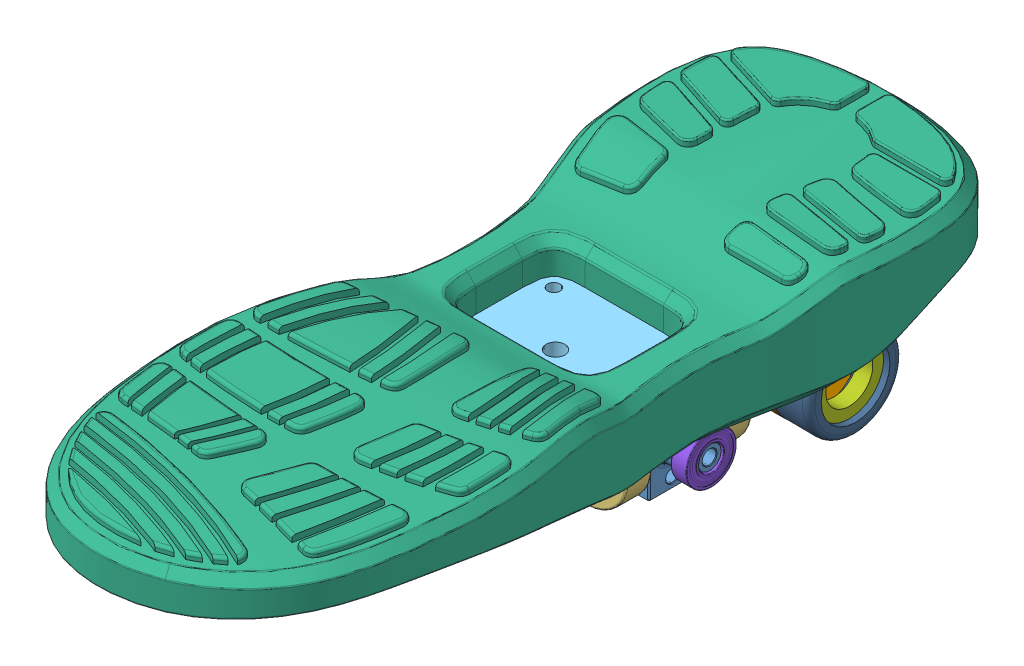
SolidWorks assembly 右小腿组件_copy, configuration 默认. Lengths in mm.
Overall size (96.41 86.26 251.7).
16 component instances, 10 part files, 7 mates.
Components (placement in the parent):
- GR1-07-2-030,踝十字轴_copy-1: GR1-07-2-030,踝十字轴_copy [默认] at (-0.0698 847.7 -0.012) x (1 0 0) z (0 0.002955 0.999996) size (38.8 29 23.8)
- GR1-07-2-033,关节延长轴_copy-1: GR1-07-2-033,关节延长轴_copy [默认] at (-0.0698 847.6409 -20.0119) x (0 0.002955 0.999996) z (-0.670955 -0.741494 0.002191) size (11 14 14)
- GR1-07-2-033,关节延长轴_copy-2: GR1-07-2-033,关节延长轴_copy [默认] at (-0.0698 847.7591 19.9879) x (0 -0.002955 -0.999996) z (0.925687 -0.378288 0.001118) size (11 14 14)
- GR1-07-2-034-G,脚板十字座_copy-1: GR1-07-2-034-G,脚板十字座_copy [默认] at (-0.0698 875.6999 -0.0947) x (0 -0.002955 -0.999996) z (-1 0 0) size (56 38 26)
- GR1-07-2-049-G,脚板转接件_copy-1: GR1-07-2-049-G,脚板转接件_copy [默认] at (-0.0698 877.7885 29.8992) x (-1 0 0) z (0 0.002955 0.999996) size (50 16 112.5)
- GR1-06-2-048,右脚包胶足撑_copy-1: GR1-06-2-048,右脚包胶足撑_copy [默认] at (-0.0698 -0.0082 -1.5321) x (1 0 0) z (0 0.002955 0.999996) size (96.41 38.94 251.59)
  - 镜向碳纤维板_copy-1: 镜向碳纤维板_copy [默认] at (0 892.7 25.025) x (1 0 0) z (0 0 -1) size (87.57 22.73 232.05)
  - 镜向硅胶脚0418_copy-1: 镜向硅胶脚0418_copy [默认] at (-885.9366 873.699 29.7166) x (-1 0 0) z (0 1 0) size (96.41 251.59 38.94)
- SC-BEAR-6802-ZZ,深沟球轴承6802_copy-3: SC-BEAR-6802-ZZ,深沟球轴承6802_copy [默认] at (9.9302 837.6311 -54.0825) x (0 -0.73398 0.679171) z (-1 0 0) size (24 24 6)
- SC-BEAR-6802-ZZ,深沟球轴承6802_copy-4: SC-BEAR-6802-ZZ,深沟球轴承6802_copy [默认] at (-5.0698 837.6311 -54.0825) x (0 -0.999638 0.026912) z (-1 0 0) size (24 24 6)
- SC-BEAR-628-8,深沟球轴承628-8_copy-5: SC-BEAR-628-8,深沟球轴承628-8_copy [默认] at (-15.0698 847.7 0.0201) x (-1 0 0) z (0 -0.426172 0.904642) size (5 16 16)
- GR1-07-2-017-G,脚板连杆座_copy-3: GR1-07-2-017-G,脚板连杆座_copy [默认] at (-35.0698 872.6352 -52.7246) x (1 0 0) z (0 -0.002955 -0.999996) size (20 40.91 30)
- GR1-07-2-059-G,脚板连杆座-1_copy-1: GR1-07-2-059-G,脚板连杆座-1_copy [默认] at (34.9302 872.6266 -55.6473) x (-1 0 0) z (0 0.002955 0.999996) size (20 40.91 30)
- SC-BEAR-628-8,深沟球轴承628-8_copy-6: SC-BEAR-628-8,深沟球轴承628-8_copy [默认] at (19.9302 847.7 -0.012) x (-1 0 0) z (0 0.991754 0.128155) size (5 16 16)
- SC-BEAR-628-8,深沟球轴承628-8_copy-7: SC-BEAR-628-8,深沟球轴承628-8_copy [默认] at (-0.0698 847.7384 12.9879) x (0 0.002955 0.999996) z (0.904136 -0.427243 0.001262) size (5 16 16)
- SC-BEAR-628-8,深沟球轴承628-8_copy-8: SC-BEAR-628-8,深沟球轴承628-8_copy [默认] at (-0.0698 847.6468 -18.0119) x (0 0.002955 0.999996) z (0.904136 -0.427243 0.001262) size (5 16 16)
Mates (geometry in assembly coordinates):
- 重合58: coincident: plane of GR1-07-2-049-G,脚板转接件_copy-1 through (-25.0698 877.7885 29.8992) normal (0 0.999996 -0.002955); plane of GR1-06-2-048,右脚包胶足撑_copy-1/镜向碳纤维板_copy-1 through (39.9302 877.8506 50.8991) normal (0 -0.999996 0.002955)
- 重合59: coincident: plane of GR1-07-2-034-G,脚板十字座_copy-1 through (-0.0698 872.6999 -0.0859) normal (0 0.999996 -0.002955); plane of GR1-07-2-049-G,脚板转接件_copy-1 through (-10.5948 872.7752 25.414) normal (0 -0.999996 0.002955)
- 重合67: coincident anti-aligned: plane of GR1-07-2-049,脚板转接件-1 through (-19.0948 863.5608 -47.1591) normal (0 -0.999996 0.002955); plane of GR1-07-2-017,脚板连杆座-3 through (-35.0698 863.5444 -52.6977) normal (0 0.999996 -0.002955)
- 重合68: coincident anti-aligned: plane of GR1-07-2-049,脚板转接件-1 through (-19.0948 863.5608 -47.1591) normal (0 -0.999996 0.002955); plane of GR1-07-2-059-G,脚板连杆座-1_copy-1 through (34.9302 863.5358 -55.6204) normal (0 0.999996 -0.002955)
- 同心82: concentric: cylinder of GR1-07-2-030,踝十字轴_copy-1 through (-0.0698 847.7263 8.888) axis (0 0.002955 0.999996) radius 4; cylinder of GR1-07-2-034-G,脚板十字座_copy-1 through (-0.0698 847.6409 -20.0119) axis (0 0.002955 0.999996) radius 7
- 同心84: concentric aligned: cylinder of SC-BEAR-6802-ZZ,深沟球轴承6802_copy-4 through (-11.0698 837.6311 -54.0825) axis (1 0 0) radius 12; cylinder of GR1-07-2-017,脚板连杆座-3 through (-10.0698 837.6311 -54.0825) axis (1 0 0) radius 12
- 重合74: coincident anti-aligned: plane of SC-BEAR-6802-ZZ,深沟球轴承6802_copy-3 through (9.9302 837.6311 -54.0825) normal (1 0 0); plane of GR1-07-2-059-G,脚板连杆座-1_copy-1 through (9.9302 837.6311 -54.0825) normal (-1 0 0)
